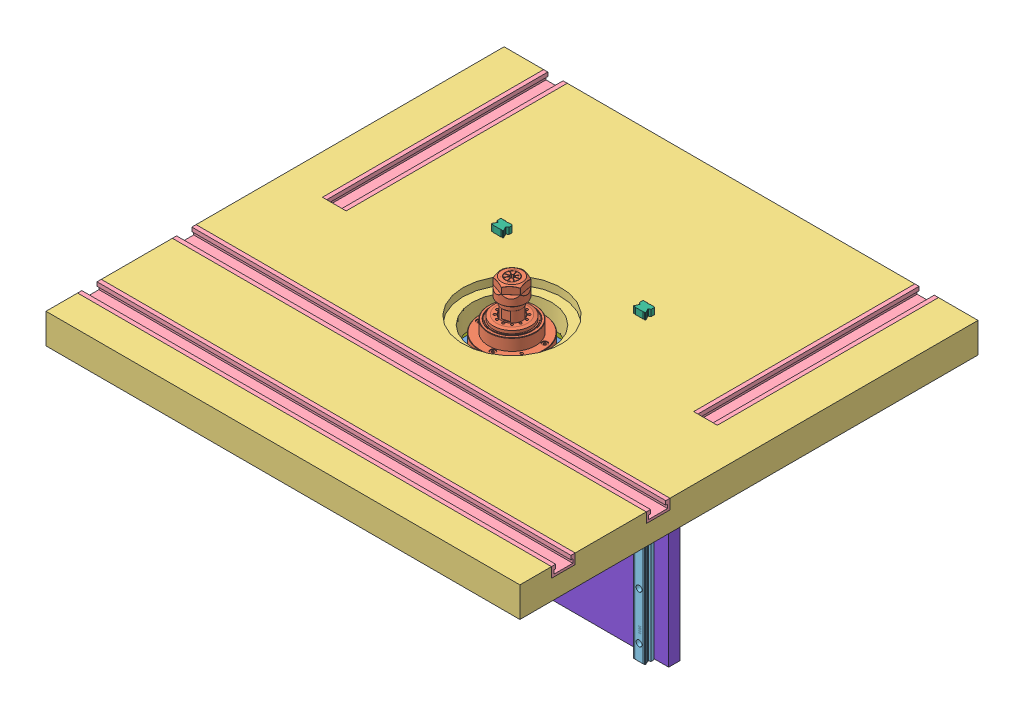
SolidWorks assembly kwrt_assy, configuration Défaut. Lengths in mm.
Overall size (600 421.51 580).
17 component instances, 8 part files, 38 mates.
Components (placement in the parent):
- spindle_support-1: spindle_support [Default] at (-224.9988 -88.0006 -343.4833) x (-1 0 0) z (0 0 -1) size (150 78 102.12)
- 2,2KW HF watercooled-1: 2,2KW HF watercooled [Défaut] at (-470.7321 15.1399 -279.2923) x (0.967116 0 -0.254336) z (0.254336 0 0.967116) size (80 298.12 80.02)
- kwrt_pt1-1: kwrt_pt1 [Défaut] at (-600 38 -580) x (1 0 0) z (0 -1 0) size (600 580 38)
- kwrt_pt2-1: kwrt_pt2 [long] at (0 25.2 -175) x (0 0 1) z (-1 0 0) size (30 12.8 600)
- kwrt_pt2-2: kwrt_pt2 [long] at (0 25.2 -55) x (0 0 1) z (-1 0 0) size (30 12.8 600)
- kwrt_pt2-3: kwrt_pt2 [short] at (-65 25.2 -580) size (30 12.8 280)
- kwrt_pt2-4: kwrt_pt2 [short] at (-535 25.2 -580) size (30 12.8 280)
- THK-SSR15-1: THK-SSR15 [預設] at (-199.6257 -170 -366.3294) x (-1 0 0) z (0 1 0) size (34 24.1 386) (flexible)
  - SSR15XWY-1-1: SSR15XWY-1 [預設] at (18.8731 -9.1039 0) size (34 24 340)
  - SSR15XWY-2-1: SSR15XWY-2 [預設] at (18.8731 -9.2039 135.9994) x (-1 0 0) z (0 0 -1) size (34 24 160)
- THK-SSR15-2: THK-SSR15 [預設] at (-379.6257 -170 -366.3294) x (-1 0 0) z (0 1 0) size (34 24.1 386) (flexible)
  - SSR15XWY-1-1: SSR15XWY-1 [預設] at (18.8731 -9.1039 0) size (34 24 340)
  - SSR15XWY-2-1: SSR15XWY-2 [預設] at (18.8731 -9.2039 135.9994) x (-1 0 0) z (0 0 -1) size (34 24 160)
- SSR15XWY-2-1: SSR15XWY-2 [預設] at (-398.4988 -124.0006 -375.5333) x (1 0 0) z (0 -1 0) size (34 24 160)
- SSR15XWY-2-2: SSR15XWY-2 [預設] at (-218.4988 -124.0006 -375.5333) x (1 0 0) z (0 -1 0) size (34 24 160)
- kwrt_pt3-1: kwrt_pt3 [Défaut] at (-198.4988 -154.0006 -343.4833) x (-1 0 0) z (0 0 -1) size (220 150 14.5)
- kwrt_pt4-1: kwrt_pt4 [Défaut] at (-193.4988 -340 -381.8833) x (-1 0 0) z (0 0 -1) size (230 340 14.5)
Mates (geometry in assembly coordinates):
- Parallèle1: parallel anti-aligned: plane of spindle_support-1 through (-225.9988 -88.0006 -343.4833) normal (0 0 -1)
- Coaxiale2: concentric anti-aligned: cylinder of spindle_support-1 through (-300 -88.0006 -290) axis (0 1 0) radius 40; cylinder of 2,2KW HF watercooled-1 through (-300 9.9894 -290) axis (0 -1 0) radius 40
- Distance2: distance = 30 mm aligned: plane of spindle_support-1 through (-300 -10.0006 -290) normal (0 1 0); plane of 2,2KW HF watercooled-1 through (-300 19.9994 -290) normal (0 1 0)
- Coïncidente1: coincident: point of kwrt_pt1-1
- Coïncidente2: coincident: line of kwrt_pt1-1 through (600 0 0) axis (0 -1 0)
- Coïncidente3: coincident: line of kwrt_pt1-1 through (0 0 -580) axis (0 0 1)
- Coïncidente4: coincident anti-aligned: plane of kwrt_pt1-1 through (-600 0 -580) normal (0 -1 0)
- Coaxiale3: concentric aligned: cylinder of 2,2KW HF watercooled-1 through (-300 9.9894 -290) axis (0 -1 0) radius 40; cylinder of kwrt_pt1-1 through (-300 38 -290) axis (0 -1 0) radius 50
- Coïncidente5: coincident anti-aligned: plane of kwrt_pt1-1 through (0 25.2 -160) normal (0 0 -1); plane of kwrt_pt2-1 through (-600 25.2 -160) normal (0 0 1)
- Coïncidente6: coincident anti-aligned: plane of kwrt_pt1-1 through (-600 25.2 -580) normal (0 1 0); plane of kwrt_pt2-1 through (-600 25.2 -190) normal (0 -1 0)
- Coïncidente7: coincident aligned: plane of kwrt_pt1-1 through (0 0 -580) normal (1 0 0); plane of kwrt_pt2-1 through (0 25.2 -175) normal (1 0 0)
- Coïncidente8: coincident anti-aligned: plane of kwrt_pt1-1 through (0 25.2 -70) normal (0 0 1); plane of kwrt_pt2-2 through (-600 25.2 -70) normal (0 0 -1)
- Coïncidente9: coincident anti-aligned: plane of kwrt_pt1-1 through (-600 25.2 -580) normal (0 1 0); plane of kwrt_pt2-2 through (-600 25.2 -70) normal (0 -1 0)
- Coïncidente10: coincident aligned: plane of kwrt_pt1-1 through (0 0 -580) normal (1 0 0); plane of kwrt_pt2-2 through (0 25.2 -55) normal (1 0 0)
- Coïncidente11: coincident anti-aligned: plane of kwrt_pt1-1 through (-600 25.2 -580) normal (0 1 0); plane of kwrt_pt2-4 through (-550 25.2 -300) normal (0 -1 0)
- Coïncidente12: coincident aligned: plane of kwrt_pt1-1 through (-600 0 -580) normal (0 0 -1); plane of kwrt_pt2-4 through (-535 25.2 -580) normal (0 0 -1)
- Coïncidente13: coincident anti-aligned: plane of kwrt_pt1-1 through (-520 25.2 -580) normal (-1 0 0); plane of kwrt_pt2-4 through (-520 25.2 -300) normal (1 0 0)
- Coïncidente14: coincident anti-aligned: plane of kwrt_pt1-1 through (-80 25.2 -580) normal (1 0 0); plane of kwrt_pt2-3 through (-80 25.2 -300) normal (-1 0 0)
- Coïncidente15: coincident anti-aligned: plane of kwrt_pt1-1 through (-600 25.2 -580) normal (0 1 0); plane of kwrt_pt2-3 through (-80 25.2 -300) normal (0 -1 0)
- Coïncidente16: coincident aligned: plane of kwrt_pt1-1 through (-600 0 -580) normal (0 0 -1); plane of kwrt_pt2-3 through (-65 25.2 -580) normal (0 0 -1)
- Coaxiale4: concentric anti-aligned: cylinder of THK-SSR15-1/SSR15XWY-2-1 through (-205.4988 -21.0006 -368.4633) axis (0 0 1) radius 1.695; cylinder of kwrt_pt3-1 through (-205.4988 -21.0006 -343.4833) axis (0 0 -1) radius 2
- Coaxiale5: concentric anti-aligned: cylinder of THK-SSR15-1/SSR15XWY-2-1 through (-231.4988 -21.0006 -368.4633) axis (0 0 1) radius 1.695; cylinder of kwrt_pt3-1 through (-231.4988 -21.0006 -343.4833) axis (0 0 -1) radius 2
- Coaxiale6: concentric anti-aligned: cylinder of SSR15XWY-2-2 through (-231.4988 -111.0006 -368.4633) axis (0 0 1) radius 1.695; cylinder of kwrt_pt3-1 through (-231.4988 -111.0006 -343.4833) axis (0 0 -1) radius 2
- Coaxiale7: concentric anti-aligned: cylinder of SSR15XWY-2-2 through (-205.4988 -137.0006 -368.4633) axis (0 0 1) radius 1.695; cylinder of kwrt_pt3-1 through (-205.4988 -137.0006 -343.4833) axis (0 0 -1) radius 2
- Coaxiale8: concentric anti-aligned: cylinder of SSR15XWY-2-1 through (-411.4988 -137.0006 -368.4633) axis (0 0 1) radius 1.695; cylinder of kwrt_pt3-1 through (-411.4988 -137.0006 -343.4833) axis (0 0 -1) radius 2
- Coaxiale9: concentric anti-aligned: cylinder of SSR15XWY-2-1 through (-385.4988 -137.0006 -368.4633) axis (0 0 1) radius 1.695; cylinder of kwrt_pt3-1 through (-385.4988 -137.0006 -343.4833) axis (0 0 -1) radius 2
- Coaxiale10: concentric anti-aligned: cylinder of THK-SSR15-2/SSR15XWY-2-1 through (-411.4988 -47.0006 -368.4633) axis (0 0 1) radius 1.695; cylinder of kwrt_pt3-1 through (-411.4988 -47.0006 -343.4833) axis (0 0 -1) radius 2
- Coaxiale11: concentric anti-aligned: cylinder of THK-SSR15-2/SSR15XWY-2-1 through (-411.4988 -21.0006 -368.4633) axis (0 0 1) radius 1.695; cylinder of kwrt_pt3-1 through (-411.4988 -21.0006 -343.4833) axis (0 0 -1) radius 2
- Coïncidente17: coincident anti-aligned: plane of THK-SSR15-2/SSR15XWY-2-1 through (-415.4988 -54.8506 -357.9833) normal (0 0 1); plane of kwrt_pt3-1 through (-198.4988 -154.0006 -357.9833) normal (0 0 -1)
- Coïncidente18: coincident anti-aligned: plane of SSR15XWY-2-1 through (-415.4988 -144.8506 -357.9833) normal (0 0 1); plane of kwrt_pt3-1 through (-198.4988 -154.0006 -357.9833) normal (0 0 -1)
- Coïncidente19: coincident anti-aligned: plane of SSR15XWY-2-2 through (-235.4988 -144.8506 -357.9833) normal (0 0 1); plane of kwrt_pt3-1 through (-198.4988 -154.0006 -357.9833) normal (0 0 -1)
- Coïncidente20: coincident anti-aligned: plane of THK-SSR15-1/SSR15XWY-2-1 through (-235.4988 -54.8506 -357.9833) normal (0 0 1); plane of kwrt_pt3-1 through (-198.4988 -154.0006 -357.9833) normal (0 0 -1)
- Coaxiale12: concentric anti-aligned: cylinder of THK-SSR15-1/SSR15XWY-1-1 through (-218.4988 -20 -381.8833) axis (0 0 1) radius 2.25; cylinder of kwrt_pt4-1 through (-218.4988 -20 -381.8833) axis (0 0 -1) radius 2.05
- Coaxiale13: concentric anti-aligned: cylinder of THK-SSR15-2/SSR15XWY-1-1 through (-398.4988 -320 -381.8833) axis (0 0 1) radius 2.25; cylinder of kwrt_pt4-1 through (-398.4988 -320 -381.8833) axis (0 0 -1) radius 2.05
- Coïncidente21: coincident anti-aligned: plane of THK-SSR15-2/SSR15XWY-1-1 through (-400.3988 0 -381.8833) normal (0 0 -1); plane of kwrt_pt4-1 through (-193.4988 -340 -381.8833) normal (0 0 1)
- Coïncidente22: coincident anti-aligned: plane of kwrt_pt1-1 through (-600 0 -580) normal (0 -1 0); plane of kwrt_pt4-1 through (-193.4988 0 -396.3833) normal (0 1 0)
- Coïncidente23: coincident anti-aligned: plane of spindle_support-1 through (-225.9988 -88.0006 -343.4833) normal (0 0 -1); plane of kwrt_pt3-1 through (-198.4988 -154.0006 -343.4833) normal (0 0 1)
- Coaxiale15: concentric aligned: cylinder of spindle_support-1 through (-363.9988 -74.0006 -343.4833) axis (0 0 1) radius 4.25; cylinder of kwrt_pt3-1 through (-363.9988 -74.0006 -357.9833) axis (0 0 1) radius 3.4
